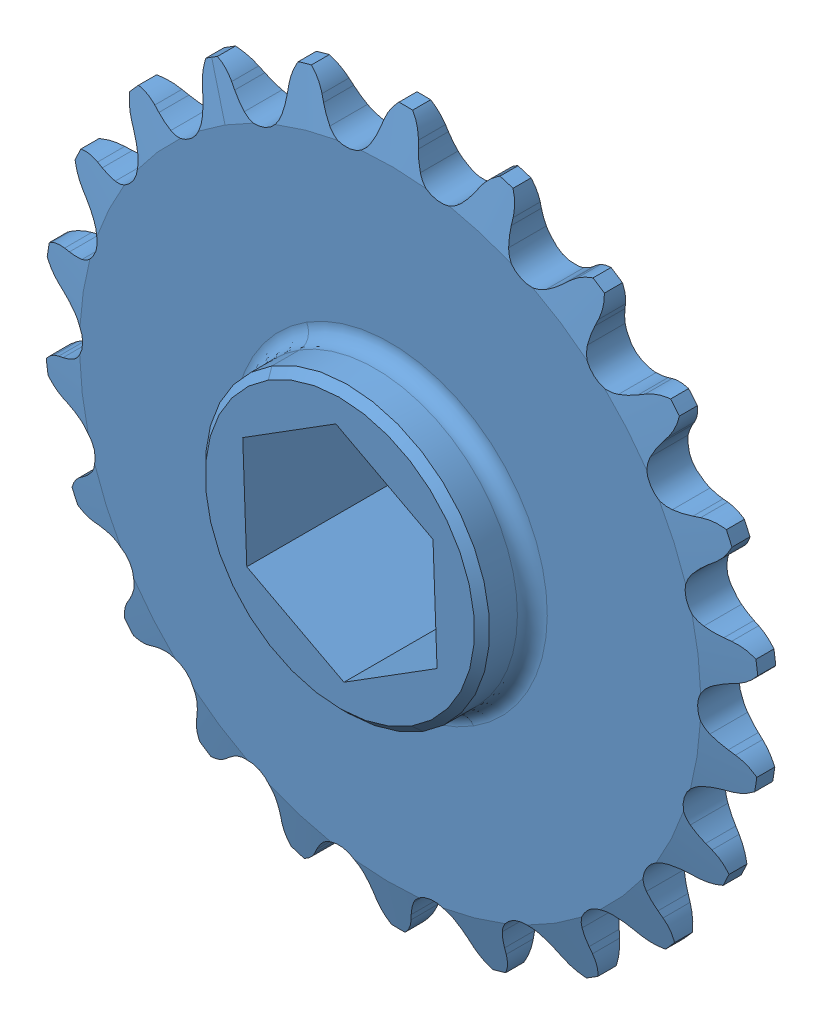
SolidWorks assembly WCP - GreyT Elevator (Cascade, 2 Stage) (1).step, configuration Default. Lengths in mm. (continued)
Components (placement in the parent): (continued)
- WCP-0326 Rev1.step-1: WCP-0326 Rev1.step [Default] at (165.1 1168.4 27.7749) x (0.127192 0.991878 0) z (0.991878 -0.127192 0) size (11.02 4.76 11) (hidden)
- WCP-0326 Rev1.step-2: WCP-0326 Rev1.step [Default] at (165.1 1193.8 27.7749) x (0.127192 0.991878 0) z (0.991878 -0.127192 0) size (11.02 4.76 11) (hidden)
- 10-32 BHCS - No Thread_WCP-0257 - 1.500.step-1: 10-32 BHCS - No Thread_WCP-0257 - 1.500.step [Default] at (101.6 1168.4 -101.6) x (-0.802481 0.596678 0) z (-0.596678 -0.802481 0) size (9.17 40.67 9.17) (hidden)
- 10-32 BHCS - No Thread_WCP-0257 - 1.500.step-2: 10-32 BHCS - No Thread_WCP-0257 - 1.500.step [Default] at (101.6 1193.8 -101.6) x (-0.802481 0.596678 0) z (-0.596678 -0.802481 0) size (9.17 40.67 9.17) (hidden)
- 10-32 BHCS - No Thread_WCP-0257 - 1.500.step-3: 10-32 BHCS - No Thread_WCP-0257 - 1.500.step [Default] at (76.2 1193.8 -101.6) x (-0.802481 0.596678 0) z (-0.596678 -0.802481 0) size (9.17 40.67 9.17) (hidden)
- 10-32 BHCS - No Thread_WCP-0257 - 1.500.step-4: 10-32 BHCS - No Thread_WCP-0257 - 1.500.step [Default] at (76.2 1168.4 -101.6) x (-0.802481 0.596678 0) z (-0.596678 -0.802481 0) size (9.17 40.67 9.17) (hidden)
- WCP-0326 Rev1.step-3: WCP-0326 Rev1.step [Default] at (101.6 1168.4 -67.4751) x (0.127192 0.991878 0) z (0.991878 -0.127192 0) size (11.02 4.76 11) (hidden)
- WCP-0326 Rev1.step-4: WCP-0326 Rev1.step [Default] at (101.6 1193.8 -67.4751) x (0.127192 0.991878 0) z (0.991878 -0.127192 0) size (11.02 4.76 11) (hidden)
- WCP-0326 Rev1.step-5: WCP-0326 Rev1.step [Default] at (76.2 1193.8 -67.4751) x (0.127192 0.991878 0) z (0.991878 -0.127192 0) size (11.02 4.76 11) (hidden)
- WCP-0326 Rev1.step-6: WCP-0326 Rev1.step [Default] at (76.2 1168.4 -67.4751) x (0.127192 0.991878 0) z (0.991878 -0.127192 0) size (11.02 4.76 11) (hidden)
- 10-32 BHCS - No Thread_WCP-0252 - 0.375.step-1: 10-32 BHCS - No Thread_WCP-0252 - 0.375.step [Default] at (165.1 11.1125 12.7) x (0.583861 0 0.811854) z (0.811854 0 -0.583861) size (9.17 12.1 9.17) (hidden)
- 10-32 BHCS - No Thread_WCP-0252 - 0.375.step-2: 10-32 BHCS - No Thread_WCP-0252 - 0.375.step [Default] at (165.1 11.1125 0) x (0.583861 0 0.811854) z (0.811854 0 -0.583861) size (9.17 12.1 9.17) (hidden)
- 10-32 BHCS - No Thread_WCP-0252 - 0.375.step-3: 10-32 BHCS - No Thread_WCP-0252 - 0.375.step [Default] at (165.1 11.1125 -12.7) x (0.583861 0 0.811854) z (0.811854 0 -0.583861) size (9.17 12.1 9.17) (hidden)
- 10-32 BHCS - No Thread_WCP-0252 - 0.375.step-4: 10-32 BHCS - No Thread_WCP-0252 - 0.375.step [Default] at (177.8 25.4 12.7) x (0 -0.948064 0.318079) z (0 0.318079 0.948064) size (9.17 12.1 9.17) (hidden)
- 10-32 BHCS - No Thread_WCP-0252 - 0.375.step-5: 10-32 BHCS - No Thread_WCP-0252 - 0.375.step [Default] at (177.8 25.4 0) x (0 -0.948064 0.318079) z (0 0.318079 0.948064) size (9.17 12.1 9.17) (hidden)
- 10-32 BHCS - No Thread_WCP-0252 - 0.375.step-6: 10-32 BHCS - No Thread_WCP-0252 - 0.375.step [Default] at (177.8 25.4 -12.7) x (0 -0.948064 0.318079) z (0 0.318079 0.948064) size (9.17 12.1 9.17) (hidden)
- 10-32 BHCS - No Thread_WCP-0252 - 0.375.step-7: 10-32 BHCS - No Thread_WCP-0252 - 0.375.step [Default] at (152.4 25.4 12.7) x (0 -0.983057 -0.183299) z (0 0.183299 -0.983057) size (9.17 12.1 9.17) (hidden)
- 10-32 BHCS - No Thread_WCP-0252 - 0.375.step-8: 10-32 BHCS - No Thread_WCP-0252 - 0.375.step [Default] at (152.4 25.4 0) x (0 -0.639879 0.768476) z (0 -0.768476 -0.639879) size (9.17 12.1 9.17) (hidden)
- 10-32 BHCS - No Thread_WCP-0252 - 0.375.step-9: 10-32 BHCS - No Thread_WCP-0252 - 0.375.step [Default] at (152.4 25.4 -12.7) x (0 -0.639879 0.768476) z (0 -0.768476 -0.639879) size (9.17 12.1 9.17) (hidden)
- 10-32 BHCS - No Thread_WCP-0252 - 0.375.step-10: 10-32 BHCS - No Thread_WCP-0252 - 0.375.step [Default] at (77.7875 50.8 -12.7) x (0 0.321661 0.946855) z (0 0.946855 -0.321661) size (9.17 12.1 9.17) (hidden)
- 10-32 BHCS - No Thread_WCP-0252 - 0.375.step-11: 10-32 BHCS - No Thread_WCP-0252 - 0.375.step [Default] at (77.7875 50.8 0) x (0 0.321661 0.946855) z (0 0.946855 -0.321661) size (9.17 12.1 9.17) (hidden)
- 10-32 BHCS - No Thread_WCP-0252 - 0.375.step-12: 10-32 BHCS - No Thread_WCP-0252 - 0.375.step [Default] at (77.7875 50.8 12.7) x (0 0.321661 0.946855) z (0 0.946855 -0.321661) size (9.17 12.1 9.17) (hidden)
- 10-32 BHCS - No Thread_WCP-0260 - 2.250.step-1: 10-32 BHCS - No Thread_WCP-0260 - 2.250.step [Default] at (76.2 1219.2 25.4) x (0.942963 -0.332897 0) z (-0.332897 -0.942963 0) size (9.17 59.72 9.17) (hidden)
- 10-32 BHCS - No Thread_WCP-0260 - 2.250.step-2: 10-32 BHCS - No Thread_WCP-0260 - 2.250.step [Default] at (101.6 1219.2 25.4) x (0.942963 -0.332897 0) z (-0.332897 -0.942963 0) size (9.17 59.72 9.17) (hidden)
- 10-32 BHCS - No Thread_WCP-0260 - 2.250.step-3: 10-32 BHCS - No Thread_WCP-0260 - 2.250.step [Default] at (76.2 25.4 25.4) x (0.942963 -0.332897 0) z (-0.332897 -0.942963 0) size (9.17 59.72 9.17) (hidden)
- 10-32 BHCS - No Thread_WCP-0260 - 2.250.step-4: 10-32 BHCS - No Thread_WCP-0260 - 2.250.step [Default] at (101.6 25.4 25.4) x (0.942963 -0.332897 0) z (-0.332897 -0.942963 0) size (9.17 59.72 9.17) (hidden)
- 10-32 BHCS - No Thread_WCP-0252 - 0.375.step-13: 10-32 BHCS - No Thread_WCP-0252 - 0.375.step [Default] at (63.5 50.8 25.4) x (0.796713 -0.604358 0) z (-0.604358 -0.796713 0) size (9.17 12.1 9.17) (hidden)
- 10-32 BHCS - No Thread_WCP-0252 - 0.375.step-14: 10-32 BHCS - No Thread_WCP-0252 - 0.375.step [Default] at (63.5 50.8 -25.4) x (-0.5764 -0.817168 0) z (0.817168 -0.5764 0) size (9.17 12.1 9.17) (hidden)
- 10-32 BHCS - No Thread_WCP-0252 - 0.375.step-15: 10-32 BHCS - No Thread_WCP-0252 - 0.375.step [Default] at (63.5 254 -25.4) x (-0.5764 -0.817168 0) z (0.817168 -0.5764 0) size (9.17 12.1 9.17) (hidden)
- 10-32 BHCS - No Thread_WCP-0252 - 0.375.step-16: 10-32 BHCS - No Thread_WCP-0252 - 0.375.step [Default] at (63.5 254 25.4) x (0.796713 -0.604358 0) z (-0.604358 -0.796713 0) size (9.17 12.1 9.17) (hidden)
- 10-32 BHCS - No Thread_WCP-0252 - 0.375.step-17: 10-32 BHCS - No Thread_WCP-0252 - 0.375.step [Default] at (77.7875 254 12.7) x (0 0.321661 0.946855) z (0 0.946855 -0.321661) size (9.17 12.1 9.17) (hidden)
- 10-32 BHCS - No Thread_WCP-0252 - 0.375.step-18: 10-32 BHCS - No Thread_WCP-0252 - 0.375.step [Default] at (77.7875 254 0) x (0 0.321661 0.946855) z (0 0.946855 -0.321661) size (9.17 12.1 9.17) (hidden)
- 10-32 BHCS - No Thread_WCP-0252 - 0.375.step-19: 10-32 BHCS - No Thread_WCP-0252 - 0.375.step [Default] at (77.7875 254 -12.7) x (0 0.321661 0.946855) z (0 0.946855 -0.321661) size (9.17 12.1 9.17) (hidden)
- 10-32 BHCS - No Thread_WCP-0252 - 0.375.step-20: 10-32 BHCS - No Thread_WCP-0252 - 0.375.step [Default] at (115.8875 1219.2 12.7) x (0 0.321661 0.946855) z (0 0.946855 -0.321661) size (9.17 12.1 9.17) (hidden)
- 10-32 BHCS - No Thread_WCP-0252 - 0.375.step-21: 10-32 BHCS - No Thread_WCP-0252 - 0.375.step [Default] at (115.8875 1219.2 0) x (0 0.321661 0.946855) z (0 0.946855 -0.321661) size (9.17 12.1 9.17) (hidden)
- 10-32 BHCS - No Thread_WCP-0252 - 0.375.step-22: 10-32 BHCS - No Thread_WCP-0252 - 0.375.step [Default] at (115.8875 1219.2 -12.7) x (0 0.321661 0.946855) z (0 0.946855 -0.321661) size (9.17 12.1 9.17) (hidden)
- 10-32 BHCS - No Thread_WCP-0252 - 0.375.step-23: 10-32 BHCS - No Thread_WCP-0252 - 0.375.step [Default] at (115.8875 25.4 -12.7) x (0 0.321661 0.946855) z (0 0.946855 -0.321661) size (9.17 12.1 9.17) (hidden)
- 10-32 BHCS - No Thread_WCP-0252 - 0.375.step-24: 10-32 BHCS - No Thread_WCP-0252 - 0.375.step [Default] at (115.8875 25.4 12.7) x (0 0.321661 0.946855) z (0 0.946855 -0.321661) size (9.17 12.1 9.17) (hidden)
- 10-32 BHCS - No Thread_WCP-0252 - 0.375.step-25: 10-32 BHCS - No Thread_WCP-0252 - 0.375.step [Default] at (115.8875 25.4 0) x (0 0.321661 0.946855) z (0 0.946855 -0.321661) size (9.17 12.1 9.17) (hidden)
- 10-32 BHCS - No Thread_WCP-0261 - 2.500.step-9: 10-32 BHCS - No Thread_WCP-0261 - 2.500.step [Default] at (38.1 25.4 25.4) x (-0.574084 -0.818796 0) z (-0.818796 0.574084 0) size (9.17 66.07 9.17) (hidden)
- 10-32 BHCS - No Thread_WCP-0261 - 2.500.step-10: 10-32 BHCS - No Thread_WCP-0261 - 2.500.step [Default] at (-50.8 25.4 25.4) x (-0.742698 -0.669626 0) z (-0.669626 0.742698 0) size (9.17 66.07 9.17) (hidden)
- 10-32 BHCS - No Thread_WCP-0261 - 2.500.step-11: 10-32 BHCS - No Thread_WCP-0261 - 2.500.step [Default] at (-38.1 25.4 25.4) x (-0.574084 -0.818796 0) z (-0.818796 0.574084 0) size (9.17 66.07 9.17) (hidden)
- 10-32 BHCS - No Thread_WCP-0261 - 2.500.step-12: 10-32 BHCS - No Thread_WCP-0261 - 2.500.step [Default] at (-25.4 25.4 25.4) x (-0.677804 -0.735243 0) z (-0.735243 0.677804 0) size (9.17 66.07 9.17) (hidden)
- WCP-0326 Rev1.step-7: WCP-0326 Rev1.step [Default] at (38.1 25.4 -31.7749) x (-0.281999 0.959415 0) z (-0.959415 -0.281999 0) size (11.02 4.76 11) (hidden)
- WCP-0326 Rev1.step-8: WCP-0326 Rev1.step [Default] at (12.7 25.4 -31.7749) x (-0.281999 0.959415 0) z (-0.959415 -0.281999 0) size (11.02 4.76 11) (hidden)
- WCP-0326 Rev1.step-9: WCP-0326 Rev1.step [Default] at (-25.4 25.4 -31.7749) x (-0.281999 0.959415 0) z (-0.959415 -0.281999 0) size (11.02 4.76 11) (hidden)
- WCP-0326 Rev1.step-10: WCP-0326 Rev1.step [Default] at (-38.1 25.4 -31.7749) x (-0.281999 0.959415 0) z (-0.959415 -0.281999 0) size (11.02 4.76 11) (hidden)
- WCP-0326 Rev1.step-11: WCP-0326 Rev1.step [Default] at (-50.8 25.4 -31.7749) x (-0.281999 0.959415 0) z (-0.959415 -0.281999 0) size (11.02 4.76 11) (hidden)
- WCP-0326 Rev1.step-12: WCP-0326 Rev1.step [Default] at (25.4 25.4 -31.7749) x (-0.281999 0.959415 0) z (-0.959415 -0.281999 0) size (11.02 4.76 11) (hidden)
- 10-32 BHCS - No Thread_WCP-0253 - 0.500.step-1: 10-32 BHCS - No Thread_WCP-0253 - 0.500.step [Default] at (-38.1 -25.4 23.114) x (0.542223 -0.840234 0) z (0.840234 0.542223 0) size (9.17 15.27 9.17) (hidden)
- 10-32 BHCS - No Thread_WCP-0253 - 0.500.step-2: 10-32 BHCS - No Thread_WCP-0253 - 0.500.step [Default] at (-12.7 -25.4 23.114) x (0.823635 -0.56712 0) z (0.56712 0.823635 0) size (9.17 15.27 9.17) (hidden)
- 10-32 BHCS - No Thread_WCP-0252 - 0.375.step-26: 10-32 BHCS - No Thread_WCP-0252 - 0.375.step [Default] at (-12.7 -11.1125 12.7) x (0.458328 0 0.888783) z (-0.888783 0 0.458328) size (9.17 12.1 9.17) (hidden)
- 10-32 BHCS - No Thread_WCP-0252 - 0.375.step-27: 10-32 BHCS - No Thread_WCP-0252 - 0.375.step [Default] at (-38.1 -11.1125 12.7) x (0.458328 0 0.888783) z (-0.888783 0 0.458328) size (9.17 12.1 9.17) (hidden)
- WCP-0326 Rev1.step-13: WCP-0326 Rev1.step [Default] at (-12.7 -17.3609 12.7) x (-0.884394 0 -0.466741) z (-0.466741 0 0.884394) size (11.02 4.76 11) (hidden)
- WCP-0326 Rev1.step-14: WCP-0326 Rev1.step [Default] at (-38.1 -17.3609 12.7) x (-0.806355 0 -0.591432) z (-0.591432 0 0.806355) size (11.02 4.76 11) (hidden)
- 10-32 BHCS - No Thread_WCP-0252 - 0.375.step-28: 10-32 BHCS - No Thread_WCP-0252 - 0.375.step [Default] at (165.1 25.4 25.4) x (0.238233 -0.971208 0) z (-0.971208 -0.238233 0) size (9.17 12.1 9.17) (hidden)
- 10-32 BHCS - No Thread_WCP-0252 - 0.375.step-29: 10-32 BHCS - No Thread_WCP-0252 - 0.375.step [Default] at (165.1 25.4 -25.4) x (0.705419 -0.708791 0) z (0.708791 0.705419 0) size (9.17 12.1 9.17) (hidden)
- #4-40 x .750L SHCS.step-1: #4-40 x .750L SHCS.step [Default] at (-4.1026 57.15 -50.8) x (0 0.222099 -0.975024) z (1 0 0) size (4.65 4.65 21.9) (hidden)
- NFS-0016_#4-40_thin_locknut_Default_As Machined_.step-1: NFS-0016_#4-40_thin_locknut_Default_As Machined_.step [Default] at (-10.35 57.15 -50.8) x (0 0.495484 -0.868617) z (0 0.868617 0.495484) size (6.37 2.79 7.35) (hidden)
- #4-40 x .750L SHCS.step-2: #4-40 x .750L SHCS.step [Default] at (-4.1026 31.75 -50.8) x (0 0.423366 0.905959) z (1 0 0) size (4.65 4.65 21.9) (hidden)
- #4-40 x .750L SHCS.step-3: #4-40 x .750L SHCS.step [Default] at (-4.1026 44.45 -50.8) x (0 -0.973772 0.227524) z (1 0 0) size (4.65 4.65 21.9) (hidden)
- NFS-0016_#4-40_thin_locknut_Default_As Machined_.step-2: NFS-0016_#4-40_thin_locknut_Default_As Machined_.step [Default] at (-10.35 44.45 -50.8) x (0 -0.910503 -0.413502) z (0 0.413502 -0.910503) size (6.37 2.79 7.35) (hidden)
- NFS-0016_#4-40_thin_locknut_Default_As Machined_.step-3: NFS-0016_#4-40_thin_locknut_Default_As Machined_.step [Default] at (-10.35 31.75 -50.8) x (0 0.495484 -0.868617) z (0 0.868617 0.495484) size (6.37 2.79 7.35) (hidden)
- 10-32 BHCS - No Thread_WCP-0261 - 2.500.step-13: 10-32 BHCS - No Thread_WCP-0261 - 2.500.step [Default] at (25.4 25.4 25.4) x (-0.992821 -0.119607 0) z (-0.119607 0.992821 0) size (9.17 66.07 9.17) (hidden)
- 10-32 BHCS - No Thread_WCP-0261 - 2.500.step-14: 10-32 BHCS - No Thread_WCP-0261 - 2.500.step [Default] at (12.7 25.4 25.4) x (-0.574084 -0.818796 0) z (-0.818796 0.574084 0) size (9.17 66.07 9.17) (hidden)
- 10-32 BHCS - No Thread_WCP-0263 - 3.000.step-1: 10-32 BHCS - No Thread_WCP-0263 - 3.000.step [Default] at (0 0 -38.1) x (0.756715 -0.653745 0) z (0.653745 0.756715 0) size (9.17 78.77 9.17) (hidden)
- 10-32 BHCS - No Thread_WCP-0263 - 3.000.step-2: 10-32 BHCS - No Thread_WCP-0263 - 3.000.step [Default] at (-50.8 0 -38.1) x (0.756715 -0.653745 0) z (0.653745 0.756715 0) size (9.17 78.77 9.17) (hidden)
- WCP-0571 Rev1.step-1: WCP-0571 Rev1.step [Default] at (-25.4 1181.1 -43.0403) size (15.88 15.88 15.71) (hidden)
- WCP-0571 Rev1.step-2: WCP-0571 Rev1.step [Default] at (-25.4 1181.1 -112.5347) x (-0.990411 -0.138152 0) z (0 0 -1) size (15.88 15.88 15.71) (hidden)
- 10-32 BHCS - No Thread_WCP-0257 - 1.500.step-5: 10-32 BHCS - No Thread_WCP-0257 - 1.500.step [Default] at (0 1181.1 -107.95) x (-0.802481 0.596678 0) z (-0.596678 -0.802481 0) size (9.17 40.67 9.17) (hidden)
- 10-32 BHCS - No Thread_WCP-0257 - 1.500.step-6: 10-32 BHCS - No Thread_WCP-0257 - 1.500.step [Default] at (-50.8 1181.1 -107.95) x (-0.853188 0.521603 0) z (-0.521603 -0.853188 0) size (9.17 40.67 9.17) (hidden)
- WCP-0560 Rev1.step-1: WCP-0560 Rev1.step [Default] at (-25.4 0 -50.8) x (-0.531612 0.846988 0) z (0 0 -1) size (47.96 47.68 9.53)
- WCP-0560 Rev1.step-2: WCP-0560 Rev1.step [Default] at (-25.4 1181.1 -50.8) x (-0.820978 -0.57096 0) z (0 0 -1) size (47.96 47.68 9.53) (hidden)
- WCP-0583-023 Rev1.step-1: WCP-0583-023 Rev1.step [Default] at (-25.4 590.55 -50.8) x (-1 0 0) z (0 0 -1) size (50.36 1231.46 9) (hidden)
- 10-32 BHCS - No Thread_WCP-0261 - 2.500.step-15: 10-32 BHCS - No Thread_WCP-0261 - 2.500.step [Default] at (-165.1 1155.7 -30.1625) x (0.802481 0.596678 0) z (-0.596678 0.802481 0) size (9.17 66.07 9.17) (hidden)
- 10-32 BHCS - No Thread_WCP-0261 - 2.500.step-16: 10-32 BHCS - No Thread_WCP-0261 - 2.500.step [Default] at (-165.1 1143 30.1625) x (-0.999937 0.011255 0) z (0.011255 0.999937 0) size (9.17 66.07 9.17) (hidden)
- WCP-EX-0019-008.step-1: WCP-EX-0019-008.step [Default] at (88.9 31.75 -50.8) size (3 1228.38 34.58) (hidden)
- WCP-0583-015 Rev1.step-1: WCP-0583-015 Rev1.step [Default] at (88.9 1181.1 -73.025) size (34.92 38.1 6.35) (hidden)
- WCP-0476 Rev1.step-1: WCP-0476 Rev1.step [Default] at (-25.4 0 -34.925) size (63.5 34.92 6.35) (hidden)
- WCP-0476 Rev1.step-2: WCP-0476 Rev1.step [Default] at (-25.4 1181.1 -73.025) size (63.5 34.92 6.35) (hidden)
- WCP-0476 Rev1.step-3: WCP-0476 Rev1.step [Default] at (-25.4 1181.1 -104.775) size (63.5 34.92 6.35) (hidden)
- WCP-0583-025 Rev1_DefaultSM-FLAT-PATTERN.step-1: WCP-0583-025 Rev1_DefaultSM-FLAT-PATTERN.step [Default] at (22.225 25.4 -29.4) x (-1 0 0) z (0 0 -1) size (44.45 50.8 31.75) (hidden)
- WCP-0583-026 Rev1.step-1: WCP-0583-026 Rev1.step [Default] at (-31.75 25.4 -29.4) x (-1 0 0) z (0 0 -1) size (50.8 50.8 31.75) (hidden)
- WCP-0207 Rev1.step-1: WCP-0207 Rev1.step [Default] at (165.1 1193.8 -50.8) x (0 0 -1) z (0.999873 -0.015939 0) size (50.8 9.5 9.5) (hidden)
- WCP-0207 Rev1.step-2: WCP-0207 Rev1.step [Default] at (165.1 1168.4 -50.8) x (0 0 -1) z (0.999873 -0.015939 0) size (50.8 9.5 9.5) (hidden)
- WCP-0308 Rev1.step-1: WCP-0308 Rev1.step [Default] at (-50.8 0 -28.575) x (0 0 -1) z (0.995626 0.093431 0) size (6.35 9.5 9.5) (hidden)
- WCP-0308 Rev1.step-2: WCP-0308 Rev1.step [Default] at (0 0 -28.575) x (0 0 -1) z (0.995626 0.093431 0) size (6.35 9.5 9.5) (hidden)
- WCP-0307 Rev1.step-1: WCP-0307 Rev1.step [Default] at (-12.7 -25.4 26.9913) x (0 0 1) z (-0.952187 0.305516 0) size (3.18 9.5 9.5) (hidden)
- WCP-0307 Rev1.step-2: WCP-0307 Rev1.step [Default] at (-38.1 -25.4 26.9913) x (0 0 1) z (-0.952187 0.305516 0) size (3.18 9.5 9.5) (hidden)
- WCP-0307 Rev1.step-3: WCP-0307 Rev1.step [Default] at (0 0 26.9913) x (0 0 1) z (-0.952187 0.305516 0) size (3.18 9.5 9.5) (hidden)
- WCP-0307 Rev1.step-4: WCP-0307 Rev1.step [Default] at (-50.8 0 26.9913) x (0 0 1) z (-0.952187 0.305516 0) size (3.18 9.5 9.5) (hidden)
- WCP-0599 Rev1.step-1: WCP-0599 Rev1.step [Default] at (-25.4 1181.1 -77.7875) x (0 0 -1) z (0.982361 -0.186992 0) size (63.5 12.67 13.72) (hidden)
- WCP-0790_500L_500_hex.step-1: WCP-0790_500L_500_hex.step [Default] at (-25.4 1181.1 -61.9125) x (0.991671 -0.128795 0) z (0 0 1) size (19.5 19.5 12.7) (hidden)
- WCP-0789_250L_500_hex.step-1: WCP-0789_250L_500_hex.step [Default] at (-25.4 0 -42.8625) size (19.5 19.5 6.35) (hidden)
- 10-32 BHCS - No Thread_WCP-0261 - 2.500.step-17: 10-32 BHCS - No Thread_WCP-0261 - 2.500.step [Default] at (-127 63.5 30.1625) x (-0.985295 -0.170861 0) z (-0.170861 0.985295 0) size (9.17 66.07 9.17) (hidden)
- 10-32 BHCS - No Thread_WCP-0261 - 2.500.step-18: 10-32 BHCS - No Thread_WCP-0261 - 2.500.step [Default] at (-127 50.8 -30.1625) x (0.742242 0.670132 0) z (-0.670132 0.742242 0) size (9.17 66.07 9.17) (hidden)
- WCP-0374 Rev1.step-1: WCP-0374 Rev1.step [Default] at (165.1 22.225 0) x (0 0 -1) z (1 0 0) size (44.07 19.05 18.67) (hidden)
- WCP-0379 Rev1.step-1: WCP-0379 Rev1.step [Default] at (165.1 22.225 0) x (0 0 -1) z (1 0 0) size (47.24 20.64 21.84) (hidden)
- WCP-0379 Rev1.step-2: WCP-0379 Rev1.step [Default] at (66.675 50.8 0) x (0 0 -1) z (0 1 0) size (47.24 20.64 21.84) (hidden)
- WCP-0374 Rev1.step-2: WCP-0374 Rev1.step [Default] at (66.675 50.8 0) x (0 0 -1) z (0 1 0) size (44.07 19.05 18.67) (hidden)
- WCP-0374 Rev1.step-3: WCP-0374 Rev1.step [Default] at (66.675 254 0) x (0 0 -1) z (0 1 0) size (44.07 19.05 18.67) (hidden)
- WCP-0379 Rev1.step-3: WCP-0379 Rev1.step [Default] at (66.675 254 0) x (0 0 -1) z (0 1 0) size (47.24 20.64 21.84) (hidden)
- WCP-0374 Rev1.step-4: WCP-0374 Rev1.step [Default] at (104.775 1219.2 0) x (0 0 -1) z (0 1 0) size (44.07 19.05 18.67) (hidden)
- WCP-0379 Rev1.step-4: WCP-0379 Rev1.step [Default] at (104.775 1219.2 0) x (0 0 -1) z (0 1 0) size (47.24 20.64 21.84) (hidden)
- WCP-0379 Rev1.step-5: WCP-0379 Rev1.step [Default] at (104.775 25.4 0) x (0 0 -1) z (0 1 0) size (47.24 20.64 21.84) (hidden)
- WCP-0374 Rev1.step-5: WCP-0374 Rev1.step [Default] at (104.775 25.4 0) x (0 0 -1) z (0 1 0) size (44.07 19.05 18.67) (hidden)
- WCP-0785_0_500_flanged_thunderhex_bearing.step-1: WCP-0785_0_500_flanged_thunderhex_bearing.step [Default] at (-25.4 0 -35.7188) x (-0.952019 0.30604 0) z (0 0 -1) size (31.12 31.12 7.94) (hidden)
- WCP-0785_0_500_flanged_thunderhex_bearing.step-2: WCP-0785_0_500_flanged_thunderhex_bearing.step [Default] at (-25.4 1181.1 -105.5688) x (-0.914179 0.405311 0) z (0 0 -1) size (31.12 31.12 7.94) (hidden)
- WCP-0785_0_500_flanged_thunderhex_bearing.step-3: WCP-0785_0_500_flanged_thunderhex_bearing.step [Default] at (-25.4 1181.1 -72.2313) x (0.656952 0.753932 0) z (0 0 1) size (31.12 31.12 7.94) (hidden)
- WCP-0800_500_hex_collar_high_strength.step-1: WCP-0800_500_hex_collar_high_strength.step [Default] at (-25.4 0 -60.325) size (28.56 28.57 9.53) (hidden)
- 10-32 BHCS - No Thread_WCP-0261 - 2.500.step-19: 10-32 BHCS - No Thread_WCP-0261 - 2.500.step [Default] at (-88.9 76.2 -30.1625) x (0.742242 0.670132 0) z (-0.670132 0.742242 0) size (9.17 66.07 9.17) (hidden)
- 10-32 BHCS - No Thread_WCP-0261 - 2.500.step-20: 10-32 BHCS - No Thread_WCP-0261 - 2.500.step [Default] at (-88.9 88.9 30.1625) x (-0.985295 -0.170861 0) z (-0.170861 0.985295 0) size (9.17 66.07 9.17) (hidden)
- 10-32 BHCS - No Thread_WCP-0261 - 2.500.step-21: 10-32 BHCS - No Thread_WCP-0261 - 2.500.step [Default] at (-88.9 228.6 30.1625) x (-0.985295 -0.170861 0) z (-0.170861 0.985295 0) size (9.17 66.07 9.17) (hidden)
- 10-32 BHCS - No Thread_WCP-0261 - 2.500.step-22: 10-32 BHCS - No Thread_WCP-0261 - 2.500.step [Default] at (-88.9 215.9 -30.1625) x (0.742242 0.670132 0) z (-0.670132 0.742242 0) size (9.17 66.07 9.17) (hidden)
- WCP-EX-0019-008.step-2: WCP-EX-0019-008.step [Default] at (-88.9 31.75 -50.8) size (3 1228.38 34.58) (hidden)
- WCP-0583-015 Rev1.step-2: WCP-0583-015 Rev1.step [Default] at (-88.9 1181.1 -73.025) x (-1 0 0) z (0 0 -1) size (34.92 38.1 6.35) (hidden)
- WCP-0326 Rev1.step-15: WCP-0326 Rev1.step [Default] at (-165.1 1193.8 27.7749) x (-0.127192 0.991878 0) z (0.991878 0.127192 0) size (11.02 4.76 11) (hidden)
- 10-32 SHCS - No Thread_WCP-0274 - 4.500.step-3: 10-32 SHCS - No Thread_WCP-0274 - 4.500.step [Default] at (-165.1 1193.8 -77.7875) x (-0.495006 -0.86889 0) z (0.86889 -0.495006 0) size (7.67 119.13 7.67) (hidden)
- WCP-0326 Rev1.step-16: WCP-0326 Rev1.step [Default] at (-165.1 1168.4 27.7749) x (-0.127192 0.991878 0) z (0.991878 0.127192 0) size (11.02 4.76 11) (hidden)
- 10-32 SHCS - No Thread_WCP-0274 - 4.500.step-4: 10-32 SHCS - No Thread_WCP-0274 - 4.500.step [Default] at (-165.1 1168.4 -77.7875) x (-0.495006 -0.86889 0) z (0.86889 -0.495006 0) size (7.67 119.13 7.67) (hidden)
- 10-32 BHCS - No Thread_WCP-0257 - 1.500.step-7: 10-32 BHCS - No Thread_WCP-0257 - 1.500.step [Default] at (-101.6 1193.8 -101.6) x (0.802481 0.596678 0) z (-0.596678 0.802481 0) size (9.17 40.67 9.17) (hidden)
- WCP-0326 Rev1.step-17: WCP-0326 Rev1.step [Default] at (-101.6 1193.8 -67.4751) x (-0.127192 0.991878 0) z (0.991878 0.127192 0) size (11.02 4.76 11) (hidden)
- 10-32 BHCS - No Thread_WCP-0257 - 1.500.step-8: 10-32 BHCS - No Thread_WCP-0257 - 1.500.step [Default] at (-101.6 1168.4 -101.6) x (0.802481 0.596678 0) z (-0.596678 0.802481 0) size (9.17 40.67 9.17) (hidden)
- WCP-0326 Rev1.step-18: WCP-0326 Rev1.step [Default] at (-101.6 1168.4 -67.4751) x (-0.127192 0.991878 0) z (0.991878 0.127192 0) size (11.02 4.76 11) (hidden)
- WCP-0326 Rev1.step-19: WCP-0326 Rev1.step [Default] at (-76.2 1168.4 -67.4751) x (-0.127192 0.991878 0) z (0.991878 0.127192 0) size (11.02 4.76 11) (hidden)
- 10-32 BHCS - No Thread_WCP-0257 - 1.500.step-9: 10-32 BHCS - No Thread_WCP-0257 - 1.500.step [Default] at (-76.2 1168.4 -101.6) x (0.802481 0.596678 0) z (-0.596678 0.802481 0) size (9.17 40.67 9.17) (hidden)
- 10-32 BHCS - No Thread_WCP-0257 - 1.500.step-10: 10-32 BHCS - No Thread_WCP-0257 - 1.500.step [Default] at (-76.2 1193.8 -101.6) x (0.802481 0.596678 0) z (-0.596678 0.802481 0) size (9.17 40.67 9.17) (hidden)
- WCP-0326 Rev1.step-20: WCP-0326 Rev1.step [Default] at (-76.2 1193.8 -67.4751) x (-0.127192 0.991878 0) z (0.991878 0.127192 0) size (11.02 4.76 11) (hidden)
- 10-32 BHCS - No Thread_WCP-0260 - 2.250.step-5: 10-32 BHCS - No Thread_WCP-0260 - 2.250.step [Default] at (-101.6 25.4 25.4) x (-0.942963 -0.332897 0) z (-0.332897 0.942963 0) size (9.17 59.72 9.17) (hidden)
- 10-32 BHCS - No Thread_WCP-0260 - 2.250.step-6: 10-32 BHCS - No Thread_WCP-0260 - 2.250.step [Default] at (-76.2 25.4 25.4) x (-0.942963 -0.332897 0) z (-0.332897 0.942963 0) size (9.17 59.72 9.17) (hidden)
- 10-32 BHCS - No Thread_WCP-0252 - 0.375.step-30: 10-32 BHCS - No Thread_WCP-0252 - 0.375.step [Default] at (-63.5 50.8 25.4) x (-0.796713 -0.604358 0) z (-0.604358 0.796713 0) size (9.17 12.1 9.17) (hidden)
- WCP-0379 Rev1.step-6: WCP-0379 Rev1.step [Default] at (-104.775 25.4 0) x (0 0 -1) z (0 -1 0) size (47.24 20.64 21.84) (hidden)
- WCP-0374 Rev1.step-6: WCP-0374 Rev1.step [Default] at (-104.775 25.4 0) x (0 0 -1) z (0 -1 0) size (44.07 19.05 18.67) (hidden)
- 10-32 BHCS - No Thread_WCP-0252 - 0.375.step-31: 10-32 BHCS - No Thread_WCP-0252 - 0.375.step [Default] at (-115.8875 25.4 0) x (0 0.321661 0.946855) z (0 -0.946855 0.321661) size (9.17 12.1 9.17) (hidden)
- 10-32 BHCS - No Thread_WCP-0252 - 0.375.step-32: 10-32 BHCS - No Thread_WCP-0252 - 0.375.step [Default] at (-115.8875 25.4 -12.7) x (0 0.321661 0.946855) z (0 -0.946855 0.321661) size (9.17 12.1 9.17) (hidden)
- 10-32 BHCS - No Thread_WCP-0252 - 0.375.step-33: 10-32 BHCS - No Thread_WCP-0252 - 0.375.step [Default] at (-115.8875 25.4 12.7) x (0 0.321661 0.946855) z (0 -0.946855 0.321661) size (9.17 12.1 9.17) (hidden)
- 10-32 BHCS - No Thread_WCP-0252 - 0.375.step-34: 10-32 BHCS - No Thread_WCP-0252 - 0.375.step [Default] at (-77.7875 50.8 0) x (0 0.321661 0.946855) z (0 -0.946855 0.321661) size (9.17 12.1 9.17) (hidden)
- 10-32 BHCS - No Thread_WCP-0252 - 0.375.step-35: 10-32 BHCS - No Thread_WCP-0252 - 0.375.step [Default] at (-77.7875 50.8 12.7) x (0 0.321661 0.946855) z (0 -0.946855 0.321661) size (9.17 12.1 9.17) (hidden)
- 10-32 BHCS - No Thread_WCP-0252 - 0.375.step-36: 10-32 BHCS - No Thread_WCP-0252 - 0.375.step [Default] at (-77.7875 50.8 -12.7) x (0 0.321661 0.946855) z (0 -0.946855 0.321661) size (9.17 12.1 9.17) (hidden)
- 10-32 BHCS - No Thread_WCP-0252 - 0.375.step-37: 10-32 BHCS - No Thread_WCP-0252 - 0.375.step [Default] at (-63.5 50.8 -25.4) x (0.5764 -0.817168 0) z (0.817168 0.5764 0) size (9.17 12.1 9.17) (hidden)
- 10-32 BHCS - No Thread_WCP-0252 - 0.375.step-38: 10-32 BHCS - No Thread_WCP-0252 - 0.375.step [Default] at (-177.8 25.4 12.7) x (0 -0.948064 0.318079) z (0 -0.318079 -0.948064) size (9.17 12.1 9.17) (hidden)
- 10-32 BHCS - No Thread_WCP-0252 - 0.375.step-39: 10-32 BHCS - No Thread_WCP-0252 - 0.375.step [Default] at (-177.8 25.4 0) x (0 -0.948064 0.318079) z (0 -0.318079 -0.948064) size (9.17 12.1 9.17) (hidden)
- 10-32 BHCS - No Thread_WCP-0252 - 0.375.step-40: 10-32 BHCS - No Thread_WCP-0252 - 0.375.step [Default] at (-177.8 25.4 -12.7) x (0 -0.948064 0.318079) z (0 -0.318079 -0.948064) size (9.17 12.1 9.17) (hidden)
- 10-32 BHCS - No Thread_WCP-0252 - 0.375.step-41: 10-32 BHCS - No Thread_WCP-0252 - 0.375.step [Default] at (-152.4 25.4 12.7) x (0 -0.983057 -0.183299) z (0 -0.183299 0.983057) size (9.17 12.1 9.17) (hidden)
- 10-32 BHCS - No Thread_WCP-0252 - 0.375.step-42: 10-32 BHCS - No Thread_WCP-0252 - 0.375.step [Default] at (-152.4 25.4 0) x (0 -0.639879 0.768476) z (0 0.768476 0.639879) size (9.17 12.1 9.17) (hidden)
- 10-32 BHCS - No Thread_WCP-0252 - 0.375.step-43: 10-32 BHCS - No Thread_WCP-0252 - 0.375.step [Default] at (-152.4 25.4 -12.7) x (0 -0.639879 0.768476) z (0 0.768476 0.639879) size (9.17 12.1 9.17) (hidden)
- WCP-0379 Rev1.step-7: WCP-0379 Rev1.step [Default] at (-165.1 22.225 0) x (0 0 -1) z (1 0 0) size (47.24 20.64 21.84) (hidden)
- WCP-0374 Rev1.step-7: WCP-0374 Rev1.step [Default] at (-165.1 22.225 0) x (0 0 -1) z (1 0 0) size (44.07 19.05 18.67) (hidden)
- 10-32 BHCS - No Thread_WCP-0252 - 0.375.step-44: 10-32 BHCS - No Thread_WCP-0252 - 0.375.step [Default] at (-165.1 11.1125 -12.7) x (-0.583861 0 0.811854) z (0.811854 0 0.583861) size (9.17 12.1 9.17) (hidden)
- 10-32 BHCS - No Thread_WCP-0252 - 0.375.step-45: 10-32 BHCS - No Thread_WCP-0252 - 0.375.step [Default] at (-165.1 11.1125 0) x (-0.583861 0 0.811854) z (0.811854 0 0.583861) size (9.17 12.1 9.17) (hidden)
- 10-32 BHCS - No Thread_WCP-0252 - 0.375.step-46: 10-32 BHCS - No Thread_WCP-0252 - 0.375.step [Default] at (-165.1 11.1125 12.7) x (-0.583861 0 0.811854) z (0.811854 0 0.583861) size (9.17 12.1 9.17) (hidden)
- 10-32 BHCS - No Thread_WCP-0252 - 0.375.step-47: 10-32 BHCS - No Thread_WCP-0252 - 0.375.step [Default] at (-63.5 254 -25.4) x (0.5764 -0.817168 0) z (0.817168 0.5764 0) size (9.17 12.1 9.17) (hidden)
- WCP-0379 Rev1.step-8: WCP-0379 Rev1.step [Default] at (-66.675 254 0) x (0 0 -1) z (0 -1 0) size (47.24 20.64 21.84) (hidden)
- WCP-0374 Rev1.step-8: WCP-0374 Rev1.step [Default] at (-66.675 254 0) x (0 0 -1) z (0 -1 0) size (44.07 19.05 18.67) (hidden)
- 10-32 BHCS - No Thread_WCP-0252 - 0.375.step-48: 10-32 BHCS - No Thread_WCP-0252 - 0.375.step [Default] at (-77.7875 254 -12.7) x (0 0.321661 0.946855) z (0 -0.946855 0.321661) size (9.17 12.1 9.17) (hidden)
- 10-32 BHCS - No Thread_WCP-0252 - 0.375.step-49: 10-32 BHCS - No Thread_WCP-0252 - 0.375.step [Default] at (-77.7875 254 0) x (0 0.321661 0.946855) z (0 -0.946855 0.321661) size (9.17 12.1 9.17) (hidden)
- 10-32 BHCS - No Thread_WCP-0252 - 0.375.step-50: 10-32 BHCS - No Thread_WCP-0252 - 0.375.step [Default] at (-77.7875 254 12.7) x (0 0.321661 0.946855) z (0 -0.946855 0.321661) size (9.17 12.1 9.17) (hidden)
- 10-32 BHCS - No Thread_WCP-0252 - 0.375.step-51: 10-32 BHCS - No Thread_WCP-0252 - 0.375.step [Default] at (-63.5 254 25.4) x (-0.796713 -0.604358 0) z (-0.604358 0.796713 0) size (9.17 12.1 9.17) (hidden)
- 10-32 BHCS - No Thread_WCP-0260 - 2.250.step-7: 10-32 BHCS - No Thread_WCP-0260 - 2.250.step [Default] at (-101.6 1219.2 25.4) x (-0.942963 -0.332897 0) z (-0.332897 0.942963 0) size (9.17 59.72 9.17) (hidden)
- 10-32 BHCS - No Thread_WCP-0260 - 2.250.step-8: 10-32 BHCS - No Thread_WCP-0260 - 2.250.step [Default] at (-76.2 1219.2 25.4) x (-0.942963 -0.332897 0) z (-0.332897 0.942963 0) size (9.17 59.72 9.17) (hidden)
- 10-32 BHCS - No Thread_WCP-0252 - 0.375.step-52: 10-32 BHCS - No Thread_WCP-0252 - 0.375.step [Default] at (-115.8875 1219.2 12.7) x (0 0.321661 0.946855) z (0 -0.946855 0.321661) size (9.17 12.1 9.17) (hidden)
- 10-32 BHCS - No Thread_WCP-0252 - 0.375.step-53: 10-32 BHCS - No Thread_WCP-0252 - 0.375.step [Default] at (-115.8875 1219.2 0) x (0 0.321661 0.946855) z (0 -0.946855 0.321661) size (9.17 12.1 9.17) (hidden)
- 10-32 BHCS - No Thread_WCP-0252 - 0.375.step-54: 10-32 BHCS - No Thread_WCP-0252 - 0.375.step [Default] at (-115.8875 1219.2 -12.7) x (0 0.321661 0.946855) z (0 -0.946855 0.321661) size (9.17 12.1 9.17) (hidden)
- WCP-0379 Rev1.step-9: WCP-0379 Rev1.step [Default] at (-104.775 1219.2 0) x (0 0 -1) z (0 -1 0) size (47.24 20.64 21.84) (hidden)
- WCP-0374 Rev1.step-9: WCP-0374 Rev1.step [Default] at (-104.775 1219.2 0) x (0 0 -1) z (0 -1 0) size (44.07 19.05 18.67) (hidden)
- WCP-0379 Rev1.step-10: WCP-0379 Rev1.step [Default] at (-66.675 50.8 0) x (0 0 -1) z (0 -1 0) size (47.24 20.64 21.84) (hidden)
- WCP-0374 Rev1.step-10: WCP-0374 Rev1.step [Default] at (-66.675 50.8 0) x (0 0 -1) z (0 -1 0) size (44.07 19.05 18.67) (hidden)
- WCP-0207 Rev1.step-3: WCP-0207 Rev1.step [Default] at (-165.1 1193.8 -50.8) x (0 0 -1) z (0.999873 0.015939 0) size (50.8 9.5 9.5) (hidden)
- WCP-0207 Rev1.step-4: WCP-0207 Rev1.step [Default] at (-165.1 1168.4 -50.8) x (0 0 -1) z (0.999873 0.015939 0) size (50.8 9.5 9.5) (hidden)
- 10-32 BHCS - No Thread_WCP-0252 - 0.375.step-55: 10-32 BHCS - No Thread_WCP-0252 - 0.375.step [Default] at (-165.1 25.4 25.4) x (-0.238233 -0.971208 0) z (-0.971208 0.238233 0) size (9.17 12.1 9.17) (hidden)
- 10-32 BHCS - No Thread_WCP-0252 - 0.375.step-56: 10-32 BHCS - No Thread_WCP-0252 - 0.375.step [Default] at (-165.1 25.4 -25.4) x (-0.705419 -0.708791 0) z (0.708791 -0.705419 0) size (9.17 12.1 9.17) (hidden)
- WCP-EX-0019-004.step-2: WCP-EX-0019-004.step [Default] at (-127 622.3 0) x (0 1 0) z (1 0 0) size (1219.2 50.8 25.4) (hidden)
- MirrorWCP-EX-0019-005.step-1: MirrorWCP-EX-0019-005.step [Default] at (-88.9 152.4 0) x (0 -1 0) z (-1 0 0) size (228.6 50.8 25.4) (hidden)
- WCP-0523 Rev1.step-1: WCP-0523 Rev1.step [Default] at (88.9 152.4 -41.6719) x (0.995786 -0.091702 0) z (-0.091702 -0.995786 0) size (15.88 0.79 15.88) (hidden)
- 10-32 BHCS - No Thread_WCP-0263 - 3.000.step-3: 10-32 BHCS - No Thread_WCP-0263 - 3.000.step [Default] at (88.9 152.4 -42.0688) x (0.163054 -0.986617 0) z (0.986617 0.163054 0) size (9.17 78.77 9.17) (hidden)
- WCP-0326 Rev1.step-21: WCP-0326 Rev1.step [Default] at (88.9 152.4 27.7749) x (0.982047 -0.188635 0) z (-0.188635 -0.982047 0) size (11.02 4.76 11) (hidden)
- WCP-0523 Rev1.step-2: WCP-0523 Rev1.step [Default] at (-88.9 152.4 -41.6719) x (0.726757 0.686895 0) z (0.686895 -0.726757 0) size (15.88 0.79 15.88) (hidden)
- WCP-0326 Rev1.step-22: WCP-0326 Rev1.step [Default] at (-88.9 152.4 27.7749) x (0.925745 -0.378148 0) z (-0.378148 -0.925745 0) size (11.02 4.76 11) (hidden)
- 10-32 BHCS - No Thread_WCP-0263 - 3.000.step-4: 10-32 BHCS - No Thread_WCP-0263 - 3.000.step [Default] at (-88.9 152.4 -42.0688) x (0.163054 -0.986617 0) z (0.986617 0.163054 0) size (9.17 78.77 9.17) (hidden)
- WCP-0203 Rev1.step-1: WCP-0203 Rev1.step [Default] at (88.9 152.4 -33.3375) x (0 0 1) z (0.991701 -0.128564 0) size (15.88 9.5 9.5) (hidden)
- WCP-0203 Rev1.step-2: WCP-0203 Rev1.step [Default] at (-88.9 152.4 -33.3375) x (0 0 1) z (-0.976351 -0.216192 0) size (15.88 9.5 9.5) (hidden)
- WCP-0583-027 Rev1.step-1: WCP-0583-027 Rev1.step [Default] at (-38.1 -12.7 25.4) x (0 -1 0) z (1 0 0) size (25.4 25.4 50.8) (hidden)
